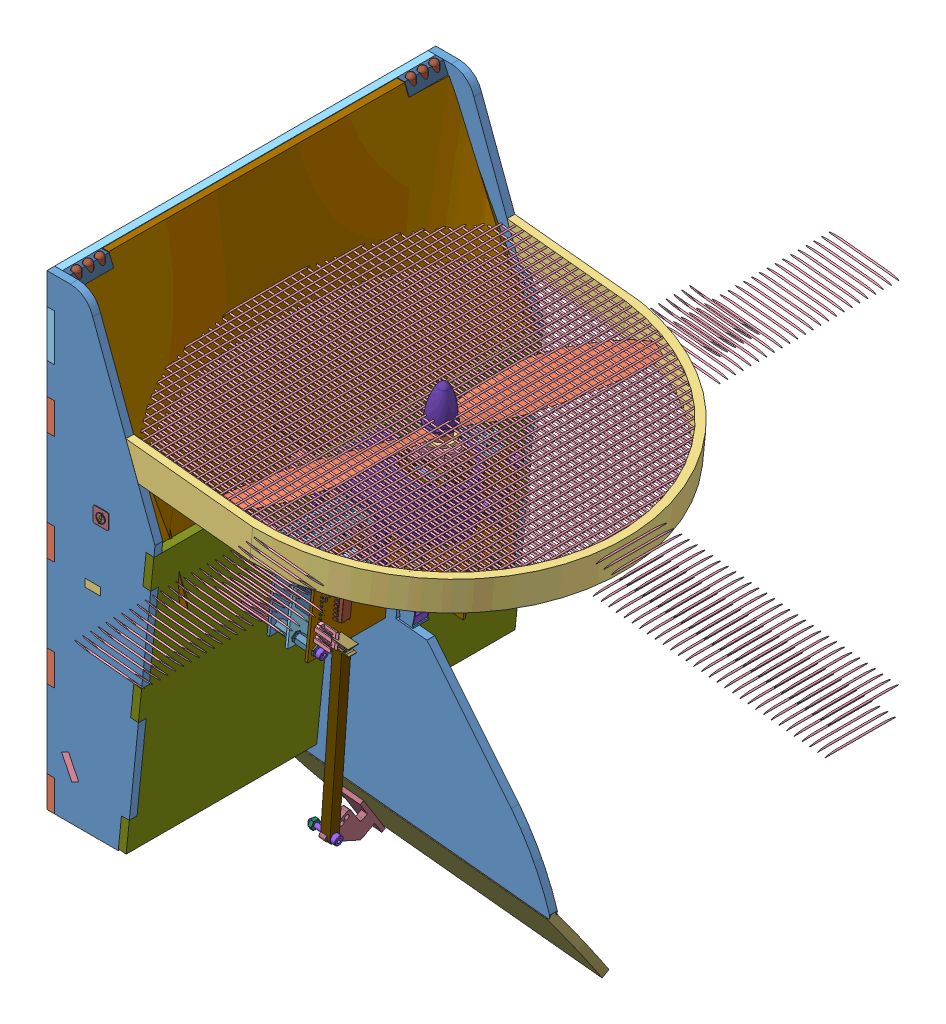
SolidWorks assembly AssTotaleSimu7, configuration Défaut. Lengths in mm. (continued)
Components (placement in the parent): (continued)
- AssStructSimu-1: AssStructSimu [Défaut] at (-125.7658 -1.8483 624.6548) x (1 0 0) z (0 0 -1) size (253.25 324.59 251.6) (continued)
  - AssCarte-1: AssCarte [Défaut] at (38.0121 147.1029 290.772) x (-0.101852 0.9948 0) z (0.9948 0.101852 0) size (66.52 130.57 98.72) (continued)
    - carte_onduleur_v3-1: carte_onduleur_v3 [Défaut] at (-131.8199 12.0892 20.7912) size (66.52 130.57 82.34) (continued)
      - U_DSPIC-1: U_DSPIC [Défaut] at (1.863 -2.61 0.803) size (7.92 35.56 7.75)
        - Open CASCADE STEP translator 6.8 1.17.1-1: Open CASCADE STEP translator 6.8 1.17.1 [Défaut] at origin size (7.92 35.56 7.75)
          - Body_1_4-1: Body_1_4 [Défaut] at (0 -0.2 4) x (1 0 0) z (0 -1 0) size (7.92 7.75 35.56)
      - C_DEC_DSPIC-1: C_DEC_DSPIC [Défaut] at (7.7 -8.8 -0.803) x (0 1 0) z (0 0 -1) size (2.34 1.04 0.5)
        - Open CASCADE STEP translator 6.8 1.6.1-1: Open CASCADE STEP translator 6.8 1.6.1 [Défaut] at origin size (2.34 1.04 0.5)
          - Body_1-1: Body_1 [Défaut] at origin size (2.29 1.04 0.43)
          - Pin_1-1: Pin_1 [Défaut] at (0.3048 0 0) x (-1 0 0) z (0 0 1) size (0.51 1.02 0.5)
          - Pin_2-1: Pin_2 [Défaut] at origin size (0.51 1.02 0.5)
      - IN-1: IN [Défaut] at (24.3 -5.3 0.803) x (0 1 0) z (0 0 1) size (10.21 15.56 26.9)
        - Open CASCADE STEP translator 6.8 1.19.1-1: Open CASCADE STEP translator 6.8 1.19.1 [Défaut] at origin size (10.21 15.56 26.9)
          - Body_1_3-1: Body_1_3 [Défaut] at (-13.5 1.8 3) x (0 1 0) z (1 0 0) size (15.56 26.9 10.21)
            - Imported-1: Imported [Défaut] at (2.0451 -4.5908 20.9802) size (8.6 15.9 10.16)
            - Imported-2: Imported [Défaut] at (-1.6683 9.1092 15.9802) x (0 0 1) z (-1 0 0) size (10.1 18.2 15.1)
              - Imported_2-1: Imported_2 [Défaut] at origin size (10.1 18.2 15.1)
              - Imported_3-1: Imported_3 [Défaut] at origin size (3.43 12.4 4.99)
              - Imported_4-1: Imported_4 [Défaut] at origin size (3.43 12.4 4.99)
              - Imported_5-1: Imported_5 [Défaut] at origin size (3.9 4.9 7)
              - Imported_6-1: Imported_6 [Défaut] at origin size (3.9 4.9 7)
              - Imported_7-1: Imported_7 [Défaut] at origin size (3.8 3.8 6.92)
              - Imported_8-1: Imported_8 [Défaut] at origin size (3.8 3.8 6.92)
              - Imported_9-1: Imported_9 [Défaut] at origin size (9 2.4 14.2)
      - CARTE_CMD-1: CARTE_CMD [Défaut] at (25 57.2 0.803) size (60.1 130 26.71)
        - Open CASCADE STEP translator 6.8 1.20.1-1: Open CASCADE STEP translator 6.8 1.20.1 [Défaut] at origin size (60.1 130 26.71)
          - Body_1_4-1: Body_1_4 [Défaut] at (-55 5 12) size (60.1 130 26.71)
            - 1_2-1: 1_2 [Défaut] at origin size (60.1 130 1.61)
            - 4-1: 4 [Défaut] at (23.6 -124.9 0.803) x (0 1 0) z (0 0 1) size (5 15.24 14.3)
              - =_[0_1_1_4]_2-1: =_[0_1_1_4]_2 [Défaut] at origin size (5 15.24 14.3)
                - 5-1: 5 [Défaut] at (0 -6.5 -13) x (0 1 0) z (0 0 -1) size (15.24 5 14.3)
            - 7-1: 7 [Défaut] at (23.6 -5 0.803) x (0 1 0) z (0 0 1) size (5 15.24 14.3)
              - =_[0_1_1_7]-1: =_[0_1_1_7] [Défaut] at origin size (5 15.24 14.3)
                - 5-1: 5 [Défaut] at (0 -6.5 -13) x (0 1 0) z (0 0 -1) size (15.24 5 14.3)
            - 10_2-1: 10_2 [Défaut] at (18.4 -115.6 0.803) size (25.4 7.92 7.75)
              - =_[0_1_1_9]-1: =_[0_1_1_9] [Défaut] at origin size (25.4 7.92 7.75)
                - 8-1: 8 [Défaut] at (11.2 4 0) x (0 1 0) z (1 0 0) size (7.92 7.75 25.4)
            - 13_2-1: 13_2 [Défaut] at (55.4 -114.7 0.803) x (-1 0 0) z (0 0 1) size (5 7.62 14.3)
              - =_[0_1_1_12]-1: =_[0_1_1_12] [Défaut] at origin size (5 7.62 14.3)
                - 11-1: 11 [Défaut] at (0 -2.5 11) x (0 -1 0) z (0 0 1) size (7.62 5 14.3)
            - 25-1: 25 [Défaut] at (56.9 -12.8 0.803) x (-1 0 0) z (0 0 1) size (16.02 47.26 11.05)
              - =_[0_1_1_15]_2-1: =_[0_1_1_15]_2 [Défaut] at origin size (16.02 47.26 11.05)
                - 23-1: 23 [Défaut] at (-36.5 21 4) x (0 -1 0) z (1 0 0) size (47.26 11.05 16.02)
                  - 14-1: 14 [Défaut] at (-7.4961 -1.5352 42.5833) size (42.58 6.55 16.01)
                  - 22-1: 22 [Défaut] at (19.3039 2.3748 37.905) x (-1 0 0) z (0 0 -1) size (10.36 6.14 15.24)
                    - 21-1: 21 [Défaut] at origin size (10.36 6.14 7.62)
                      - 19_2-1: 19_2 [Défaut] at origin size (10.36 6.14 2.54)
                        - 15-1: 15 [Défaut] at origin size (8.4 2.54 2.54)
                        - 16-1: 16 [Défaut] at (-0.0461 1.2682 1.27) x (0 0 -1) z (0.999998 -0.002105 0) size (1.95 5.07 7.58)
                      - 19_2-2: 19_2 [Défaut] at (0 0 -2.54) size (10.36 6.14 2.54)
                        - 15-1: 15 [Défaut] at origin size (8.4 2.54 2.54)
                        - 16-1: 16 [Défaut] at (-0.0461 1.2682 1.27) x (0 0 -1) z (0.999998 -0.002105 0) size (1.95 5.07 7.58)
                      - 19_2-3: 19_2 [Défaut] at (0 0 -5.08) size (10.36 6.14 2.54)
                        - 15-1: 15 [Défaut] at origin size (8.4 2.54 2.54)
                        - 16-1: 16 [Défaut] at (-0.0461 1.2682 1.27) x (0 0 -1) z (0.999998 -0.002105 0) size (1.95 5.07 7.58)
                    - 21-2: 21 [Défaut] at (0 0 -7.62) size (10.36 6.14 7.62)
                      - 19_2-1: 19_2 [Défaut] at origin size (10.36 6.14 2.54)
                        - 15-1: 15 [Défaut] at origin size (8.4 2.54 2.54)
                        - 16-1: 16 [Défaut] at (-0.0461 1.2682 1.27) x (0 0 -1) z (0.999998 -0.002105 0) size (1.95 5.07 7.58)
                      - 19_2-2: 19_2 [Défaut] at (0 0 -2.54) size (10.36 6.14 2.54)
                        - 15-1: 15 [Défaut] at origin size (8.4 2.54 2.54)
                        - 16-1: 16 [Défaut] at (-0.0461 1.2682 1.27) x (0 0 -1) z (0.999998 -0.002105 0) size (1.95 5.07 7.58)
                      - 19_2-3: 19_2 [Défaut] at (0 0 -5.08) size (10.36 6.14 2.54)
                        - 15-1: 15 [Défaut] at origin size (8.4 2.54 2.54)
                        - 16-1: 16 [Défaut] at (-0.0461 1.2682 1.27) x (0 0 -1) z (0.999998 -0.002105 0) size (1.95 5.07 7.58)
            - 31-1: 31 [Défaut] at (12.9 -104.5 0.803) size (6.76 3.64 4.37)
              - =_[0_1_1_24]-1: =_[0_1_1_24] [Défaut] at origin size (6.76 3.64 4.37)
                - 29-1: 29 [Défaut] at (-0.3 -2 0) size (6.76 3.64 4.37)
                  - =_[0_1_1_3]_3-1: =_[0_1_1_3]_3 [Défaut] at origin size (6 3.64 4.37)
                  - =_[0_1_1_4]_3-1: =_[0_1_1_4]_3 [Défaut] at origin size (0.38 1 0.67)
                  - =_[0_1_1_5]_3-1: =_[0_1_1_5]_3 [Défaut] at origin size (0.38 1 0.67)
            - 36-1: 36 [Défaut] at (28.6 -12.2 0.803) x (0 -1 0) z (0 0 1) size (2.34 1.04 0.5)
              - =_[0_1_1_30]-1: =_[0_1_1_30] [Défaut] at origin size (2.34 1.04 0.5)
                - 32_2-1: 32_2 [Défaut] at origin size (2.29 1.04 0.43)
                - 33_2-1: 33_2 [Défaut] at (0.3048 0 0) x (-1 0 0) z (0 0 1) size (0.51 1.02 0.5)
                - 34-1: 34 [Défaut] at origin size (0.51 1.02 0.5)
            - 38-1: 38 [Défaut] at (23.7 -12.2 0.803) x (0 -1 0) z (0 0 1) size (2.34 1.04 0.5)
              - =_[0_1_1_30]-1: =_[0_1_1_30] [Défaut] at origin size (2.34 1.04 0.5)
                - 32_2-1: 32_2 [Défaut] at origin size (2.29 1.04 0.43)
                - 33_2-1: 33_2 [Défaut] at (0.3048 0 0) x (-1 0 0) z (0 0 1) size (0.51 1.02 0.5)
                - 34-1: 34 [Défaut] at origin size (0.51 1.02 0.5)
            - 40_2-1: 40_2 [Défaut] at (26.2 -12.2 0.803) x (0 -1 0) z (0 0 1) size (2.34 1.04 0.5)
              - =_[0_1_1_30]-1: =_[0_1_1_30] [Défaut] at origin size (2.34 1.04 0.5)
                - 32_2-1: 32_2 [Défaut] at origin size (2.29 1.04 0.43)
                - 33_2-1: 33_2 [Défaut] at (0.3048 0 0) x (-1 0 0) z (0 0 1) size (0.51 1.02 0.5)
                - 34-1: 34 [Défaut] at origin size (0.51 1.02 0.5)
            - 42_2-1: 42_2 [Défaut] at (24.4 -119.2 0.803) size (2.34 1.04 0.5)
              - =_[0_1_1_30]-1: =_[0_1_1_30] [Défaut] at origin size (2.34 1.04 0.5)
                - 32_2-1: 32_2 [Défaut] at origin size (2.29 1.04 0.43)
                - 33_2-1: 33_2 [Défaut] at (0.3048 0 0) x (-1 0 0) z (0 0 1) size (0.51 1.02 0.5)
                - 34-1: 34 [Défaut] at origin size (0.51 1.02 0.5)
            - 45-1: 45 [Défaut] at (46.4 -125 0.803) size (5.08 5 14.3)
              - =_[0_1_1_38]-1: =_[0_1_1_38] [Défaut] at origin size (5.08 5 14.3)
                - 46-1: 46 [Défaut] at (1.2 0 11) size (5.08 5 14.3)
            - 48-1: 48 [Défaut] at (40.1 -125 0.803) size (5.08 5 14.3)
              - =_[0_1_1_41]-1: =_[0_1_1_41] [Défaut] at origin size (5.08 5 14.3)
                - 46-1: 46 [Défaut] at (1.2 0 11) size (5.08 5 14.3)
            - 51-1: 51 [Défaut] at (6.4 -119.9 0.803) x (0 1 0) z (0 0 1) size (15.24 2.54 7.37)
              - =_[0_1_1_43]-1: =_[0_1_1_43] [Défaut] at origin size (15.24 2.54 7.37)
                - 49_2-1: 49_2 [Défaut] at (6.5 0 0) x (1 0 0) z (0 -1 0) size (15.24 7.37 2.54)
            - 57_2-1: 57_2 [Défaut] at (50.8796 -121.1 -0.803) x (-1 0 0) z (0 0 -1) size (2.54 1.98 0.64)
              - =_[0_1_1_46]-1: =_[0_1_1_46] [Défaut] at origin size (2.54 1.98 0.64)
                - 52-1: 52 [Défaut] at origin size (2.54 1.14 0.58)
                - 53-1: 53 [Défaut] x (0 -1 0) z (0 0 1) size (0.43 0.51 0.38)
                - 54-1: 54 [Défaut] at (1.8796 1.8796 0) x (0 -1 0) z (0 0 1) size (0.43 0.51 0.38)
                - 55-1: 55 [Défaut] at (-0.9652 -2.8448 0) x (0 1 0) z (0 0 1) size (0.41 0.51 0.38)
            - 59_2-1: 59_2 [Défaut] at (43.6398 -120.995 -0.803) x (-1 0 0) z (0 0 -1) size (2.54 1.98 0.64)
              - =_[0_1_1_46]-1: =_[0_1_1_46] [Défaut] at origin size (2.54 1.98 0.64)
                - 52-1: 52 [Défaut] at origin size (2.54 1.14 0.58)
                - 53-1: 53 [Défaut] x (0 -1 0) z (0 0 1) size (0.43 0.51 0.38)
                - 54-1: 54 [Défaut] at (1.8796 1.8796 0) x (0 -1 0) z (0 0 1) size (0.43 0.51 0.38)
                - 55-1: 55 [Défaut] at (-0.9652 -2.8448 0) x (0 1 0) z (0 0 1) size (0.41 0.51 0.38)
            - 61_2-1: 61_2 [Défaut] at (47.6 -119.9 -0.803) x (-1 0 0) z (0 0 -1) size (2.34 1.04 0.5)
              - =_[0_1_1_30]-1: =_[0_1_1_30] [Défaut] at origin size (2.34 1.04 0.5)
                - 32_2-1: 32_2 [Défaut] at origin size (2.29 1.04 0.43)
                - 33_2-1: 33_2 [Défaut] at (0.3048 0 0) x (-1 0 0) z (0 0 1) size (0.51 1.02 0.5)
                - 34-1: 34 [Défaut] at origin size (0.51 1.02 0.5)
            - 63-1: 63 [Défaut] at (40.4 -119.9 -0.803) x (-1 0 0) z (0 0 -1) size (2.34 1.04 0.5)
              - =_[0_1_1_30]-1: =_[0_1_1_30] [Défaut] at origin size (2.34 1.04 0.5)
                - 32_2-1: 32_2 [Défaut] at origin size (2.29 1.04 0.43)
                - 33_2-1: 33_2 [Défaut] at (0.3048 0 0) x (-1 0 0) z (0 0 1) size (0.51 1.02 0.5)
                - 34-1: 34 [Défaut] at origin size (0.51 1.02 0.5)
            - 68-1: 68 [Défaut] at (47.7 -21.8 -0.803) x (0 1 0) z (0 0 -1) size (2.34 1.04 0.5)
              - =_[0_1_1_55]-1: =_[0_1_1_55] [Défaut] at origin size (2.34 1.04 0.5)
                - 64-1: 64 [Défaut] at origin size (2.29 1.04 0.43)
                - 65-1: 65 [Défaut] at (0.3048 0 0) x (-1 0 0) z (0 0 1) size (0.51 1.02 0.5)
                - 66-1: 66 [Défaut] at origin size (0.51 1.02 0.5)
            - 70-1: 70 [Défaut] at (47.6 -121.7 -0.803) x (-1 0 0) z (0 0 -1) size (2.34 1.04 0.5)
              - =_[0_1_1_30]-1: =_[0_1_1_30] [Défaut] at origin size (2.34 1.04 0.5)
                - 32_2-1: 32_2 [Défaut] at origin size (2.29 1.04 0.43)
                - 33_2-1: 33_2 [Défaut] at (0.3048 0 0) x (-1 0 0) z (0 0 1) size (0.51 1.02 0.5)
                - 34-1: 34 [Défaut] at origin size (0.51 1.02 0.5)
            - 72_2-1: 72_2 [Défaut] at (40.4 -121.5 -0.803) x (-1 0 0) z (0 0 -1) size (2.34 1.04 0.5)
              - =_[0_1_1_30]-1: =_[0_1_1_30] [Défaut] at origin size (2.34 1.04 0.5)
                - 32_2-1: 32_2 [Défaut] at origin size (2.29 1.04 0.43)
                - 33_2-1: 33_2 [Défaut] at (0.3048 0 0) x (-1 0 0) z (0 0 1) size (0.51 1.02 0.5)
                - 34-1: 34 [Défaut] at origin size (0.51 1.02 0.5)
            - 74_2-1: 74_2 [Défaut] at (47.7 -18.3 -0.803) x (0 1 0) z (0 0 -1) size (2.34 1.04 0.5)
              - =_[0_1_1_55]-1: =_[0_1_1_55] [Défaut] at origin size (2.34 1.04 0.5)
                - 64-1: 64 [Défaut] at origin size (2.29 1.04 0.43)
                - 65-1: 65 [Défaut] at (0.3048 0 0) x (-1 0 0) z (0 0 1) size (0.51 1.02 0.5)
                - 66-1: 66 [Défaut] at origin size (0.51 1.02 0.5)
            - 76_2-1: 76_2 [Défaut] at (45.5 -118.3 -0.803) x (1 0 0) z (0 0 -1) size (2.34 1.04 0.5)
              - =_[0_1_1_30]-1: =_[0_1_1_30] [Défaut] at origin size (2.34 1.04 0.5)
                - 32_2-1: 32_2 [Défaut] at origin size (2.29 1.04 0.43)
                - 33_2-1: 33_2 [Défaut] at (0.3048 0 0) x (-1 0 0) z (0 0 1) size (0.51 1.02 0.5)
                - 34-1: 34 [Défaut] at origin size (0.51 1.02 0.5)
            - 78_2-1: 78_2 [Défaut] at (38.2 -118.3 -0.803) x (1 0 0) z (0 0 -1) size (2.34 1.04 0.5)
              - =_[0_1_1_30]-1: =_[0_1_1_30] [Défaut] at origin size (2.34 1.04 0.5)
                - 32_2-1: 32_2 [Défaut] at origin size (2.29 1.04 0.43)
                - 33_2-1: 33_2 [Défaut] at (0.3048 0 0) x (-1 0 0) z (0 0 1) size (0.51 1.02 0.5)
                - 34-1: 34 [Défaut] at origin size (0.51 1.02 0.5)
            - 80_2-1: 80_2 [Défaut] at (28.6 -10.7 0.803) x (0 1 0) z (0 0 1) size (2.34 1.04 0.5)
              - =_[0_1_1_55]-1: =_[0_1_1_55] [Défaut] at origin size (2.34 1.04 0.5)
                - 64-1: 64 [Défaut] at origin size (2.29 1.04 0.43)
                - 65-1: 65 [Défaut] at (0.3048 0 0) x (-1 0 0) z (0 0 1) size (0.51 1.02 0.5)
                - 66-1: 66 [Défaut] at origin size (0.51 1.02 0.5)
            - 82_2-1: 82_2 [Défaut] at (23.7 -10.7 0.803) x (0 1 0) z (0 0 1) size (2.34 1.04 0.5)
              - =_[0_1_1_55]-1: =_[0_1_1_55] [Défaut] at origin size (2.34 1.04 0.5)
                - 64-1: 64 [Défaut] at origin size (2.29 1.04 0.43)
                - 65-1: 65 [Défaut] at (0.3048 0 0) x (-1 0 0) z (0 0 1) size (0.51 1.02 0.5)
                - 66-1: 66 [Défaut] at origin size (0.51 1.02 0.5)
            - 84-1: 84 [Défaut] at (26.2 -10.7 0.803) x (0 1 0) z (0 0 1) size (2.34 1.04 0.5)
              - =_[0_1_1_55]-1: =_[0_1_1_55] [Défaut] at origin size (2.34 1.04 0.5)
                - 64-1: 64 [Défaut] at origin size (2.29 1.04 0.43)
                - 65-1: 65 [Défaut] at (0.3048 0 0) x (-1 0 0) z (0 0 1) size (0.51 1.02 0.5)
                - 66-1: 66 [Défaut] at origin size (0.51 1.02 0.5)
            - 86-1: 86 [Défaut] at (23.0336 -119.2 0.803) x (-1 0 0) z (0 0 1) size (2.34 1.04 0.5)
              - =_[0_1_1_55]-1: =_[0_1_1_55] [Défaut] at origin size (2.34 1.04 0.5)
                - 64-1: 64 [Défaut] at origin size (2.29 1.04 0.43)
                - 65-1: 65 [Défaut] at (0.3048 0 0) x (-1 0 0) z (0 0 1) size (0.51 1.02 0.5)
                - 66-1: 66 [Défaut] at origin size (0.51 1.02 0.5)
            - 88-1: 88 [Défaut] at (14.1 -114.2 0.803) x (0 -1 0) z (0 0 1) size (2.34 1.04 0.5)
              - =_[0_1_1_55]-1: =_[0_1_1_55] [Défaut] at origin size (2.34 1.04 0.5)
                - 64-1: 64 [Défaut] at origin size (2.29 1.04 0.43)
                - 65-1: 65 [Défaut] at (0.3048 0 0) x (-1 0 0) z (0 0 1) size (0.51 1.02 0.5)
                - 66-1: 66 [Défaut] at origin size (0.51 1.02 0.5)
            - 90-1: 90 [Défaut] at (43.6 -107.8 -0.803) x (1 0 0) z (0 0 -1) size (2.34 1.04 0.5)
              - =_[0_1_1_55]-1: =_[0_1_1_55] [Défaut] at origin size (2.34 1.04 0.5)
                - 64-1: 64 [Défaut] at origin size (2.29 1.04 0.43)
                - 65-1: 65 [Défaut] at (0.3048 0 0) x (-1 0 0) z (0 0 1) size (0.51 1.02 0.5)
                - 66-1: 66 [Défaut] at origin size (0.51 1.02 0.5)
            - 92-1: 92 [Défaut] at (43.6 -106 -0.803) x (1 0 0) z (0 0 -1) size (2.34 1.04 0.5)
              - =_[0_1_1_55]-1: =_[0_1_1_55] [Défaut] at origin size (2.34 1.04 0.5)
                - 64-1: 64 [Défaut] at origin size (2.29 1.04 0.43)
                - 65-1: 65 [Défaut] at (0.3048 0 0) x (-1 0 0) z (0 0 1) size (0.51 1.02 0.5)
                - 66-1: 66 [Défaut] at origin size (0.51 1.02 0.5)
            - 175-1: 175 [Défaut] at (10 -21.7 0.803) x (0 -1 0) z (0 0 1) size (15 25.4 12.78)
              - =_[0_1_1_72]-1: =_[0_1_1_72] [Défaut] at origin size (15 25.4 12.78)
                - 173-1: 173 [Défaut] at (-1.4 -1 12) x (-1 0 0) z (0 1 0) size (15 12.78 25.4)
                  - board_1-1: board_1 [Défaut] at (-7.5 -1.57 12.5) size (15 1.57 25)
                  - hole_plating_20-1: hole_plating_20 [Défaut] at (-1.5 0 23.93) size (1.5 0.01 1.5)
                  - hole_plating_20-2: hole_plating_20 [Défaut] at (-1.5 0 21.39) size (1.5 0.01 1.5)
                  - hole_plating_20-3: hole_plating_20 [Défaut] at (-1.5 0 8.69) size (1.5 0.01 1.5)
                  - hole_plating_20-4: hole_plating_20 [Défaut] at (-1.5 -1.58 13.77) size (1.5 0.01 1.5)
                  - hole_plating_20-5: hole_plating_20 [Défaut] at (-1.5 0 16.31) size (1.5 0.01 1.5)
                  - hole_plating_20-6: hole_plating_20 [Défaut] at (-1.5 0 18.85) size (1.5 0.01 1.5)
                  - hole_plating_20-7: hole_plating_20 [Défaut] at (-1.5 0 13.77) size (1.5 0.01 1.5)
                  - hole_plating_20-8: hole_plating_20 [Défaut] at (-1.5 -1.58 11.23) size (1.5 0.01 1.5)
                  - hole_plating_20-9: hole_plating_20 [Défaut] at (-1.5 -1.58 18.85) size (1.5 0.01 1.5)
                  - hole_plating_20-10: hole_plating_20 [Défaut] at (-1.5 -1.58 6.15) size (1.5 0.01 1.5)
                  - hole_plating_20-11: hole_plating_20 [Défaut] at (-1.5 0 1.07) size (1.5 0.01 1.5)
                  - hole_plating_20-12: hole_plating_20 [Défaut] at (-1.5 -1.58 3.61) size (1.5 0.01 1.5)
                  - hole_plating_20-13: hole_plating_20 [Défaut] at (-1.5 -1.58 1.07) size (1.5 0.01 1.5)
                  - hole_plating_20-14: hole_plating_20 [Défaut] at (-1.5 -1.58 8.69) size (1.5 0.01 1.5)
                  - hole_plating_20-15: hole_plating_20 [Défaut] at (-1.5 -1.58 16.31) size (1.5 0.01 1.5)
                  - hole_plating_20-16: hole_plating_20 [Défaut] at (-1.5 0 11.23) size (1.5 0.01 1.5)
                  - hole_plating_20-17: hole_plating_20 [Défaut] at (-1.5 0 3.61) size (1.5 0.01 1.5)
                  - hole_plating_20-18: hole_plating_20 [Défaut] at (-1.5 -1.58 21.39) size (1.5 0.01 1.5)
                  - hole_plating_20-19: hole_plating_20 [Défaut] at (-1.5 0 6.15) size (1.5 0.01 1.5)
                  - hole_plating_20-20: hole_plating_20 [Défaut] at (-1.5 -1.58 23.93) size (1.5 0.01 1.5)
                  - Pin_Header_1x10_TH_Pitch_2.54mm_1-1: Pin_Header_1x10_TH_Pitch_2.54mm_1 [Défaut] at (-1.5 -1.5786 23.93) x (0 0 -1) z (0 -1 0) size (25.4 2.54 12.7)
                    - 124-1: 124 [Défaut] at origin size (25.4 2.54 2.8)
                      - =_[0_1_1_77]-1: =_[0_1_1_77] [Défaut] at origin size (2.54 2.54 2.8)
                      - =_[0_1_1_79]-1: =_[0_1_1_79] [Défaut] at origin size (2.54 2.54 2.8)
                      - =_[0_1_1_80]-1: =_[0_1_1_80] [Défaut] at origin size (2.54 2.54 2.8)
                      - =_[0_1_1_81]-1: =_[0_1_1_81] [Défaut] at origin size (2.54 2.54 2.8)
                      - =_[0_1_1_82]-1: =_[0_1_1_82] [Défaut] at origin size (2.54 2.54 2.8)
                      - =_[0_1_1_83]-1: =_[0_1_1_83] [Défaut] at origin size (2.54 2.54 2.8)
                      - =_[0_1_1_84]-1: =_[0_1_1_84] [Défaut] at origin size (2.54 2.54 2.8)
                      - =_[0_1_1_85]-1: =_[0_1_1_85] [Défaut] at origin size (2.54 2.54 2.8)
                      - =_[0_1_1_86]-1: =_[0_1_1_86] [Défaut] at origin size (2.54 2.54 2.8)
                      - =_[0_1_1_87]-1: =_[0_1_1_87] [Défaut] at origin size (2.54 2.54 2.8)
                    - 135-1: 135 [Défaut] at origin size (23.49 0.63 12.7)
                      - =_[0_1_1_88]-1: =_[0_1_1_88] [Défaut] at origin size (0.63 0.63 12.7)
                      - =_[0_1_1_90]-1: =_[0_1_1_90] [Défaut] at origin size (0.63 0.63 12.7)
                      - =_[0_1_1_91]-1: =_[0_1_1_91] [Défaut] at origin size (0.63 0.63 12.7)
                      - =_[0_1_1_92]-1: =_[0_1_1_92] [Défaut] at origin size (0.63 0.63 12.7)
                      - =_[0_1_1_93]-1: =_[0_1_1_93] [Défaut] at origin size (0.63 0.63 12.7)
                      - =_[0_1_1_94]-1: =_[0_1_1_94] [Défaut] at origin size (0.63 0.63 12.7)
                      - =_[0_1_1_95]-1: =_[0_1_1_95] [Défaut] at origin size (0.63 0.63 12.7)
                      - =_[0_1_1_96]-1: =_[0_1_1_96] [Défaut] at origin size (0.63 0.63 12.7)
                      - =_[0_1_1_97]-1: =_[0_1_1_97] [Défaut] at origin size (0.63 0.63 12.7)
                      - =_[0_1_1_98]-1: =_[0_1_1_98] [Défaut] at origin size (0.63 0.63 12.7)
                  - MPU-9250_1-1: MPU-9250_1 [Défaut] at (-8 0.05 12.5) x (-1 0 0) z (0 1 0) size (3 3 1.05)
                  - tantalum_10uF_1-1: tantalum_10uF_1 [Défaut] at (-13.167 0.1 10.9372) x (0 0 1) z (0 1 0) size (3.4 1.6 1.71)
                  - SOT23_5_1-1: SOT23_5_1 [Défaut] at (-7.475 -0.0136 21) x (0 0 1) z (0 1 0) size (3 3.2 0.92)
                  - RESC-0603_5-1: RESC-0603_5 [Défaut] at (-6.85 0 7.45) x (1 0 0) z (0 1 0) size (1.7 0.9 0.55)
                    - 143-1: 143 [Défaut] at origin size (1.7 0.9 0.55)
                      - =_[0_1_1_103]-1: =_[0_1_1_103] [Défaut] at origin size (0.4 0.9 0.53)
                      - =_[0_1_1_105]-1: =_[0_1_1_105] [Défaut] at origin size (0.4 0.9 0.53)
                      - =_[0_1_1_106]-1: =_[0_1_1_106] [Défaut] at origin size (1.64 0.9 0.52)
                    - 152-1: 152 [Défaut] at origin
                      - =_[0_1_1_107]-1: =_[0_1_1_107] [Défaut] at origin
                      - =_[0_1_1_109]-1: =_[0_1_1_109] [Défaut] at origin
                      - =_[0_1_1_110]-1: =_[0_1_1_110] [Défaut] at origin
                      - =_[0_1_1_111]-1: =_[0_1_1_111] [Défaut] at origin
                      - =_[0_1_1_112]-1: =_[0_1_1_112] [Défaut] at origin
                      - =_[0_1_1_113]-1: =_[0_1_1_113] [Défaut] at origin
                      - =_[0_1_1_114]-1: =_[0_1_1_114] [Défaut] at origin
                      - =_[0_1_1_115]-1: =_[0_1_1_115] [Défaut] at origin
                  - RESC-0603_5-2: RESC-0603_5 [Défaut] at (-9.85 0 16.05) x (1 0 0) z (0 1 0) size (1.7 0.9 0.55)
                    - 143-1: 143 [Défaut] at origin size (1.7 0.9 0.55)
                      - =_[0_1_1_103]-1: =_[0_1_1_103] [Défaut] at origin size (0.4 0.9 0.53)
                      - =_[0_1_1_105]-1: =_[0_1_1_105] [Défaut] at origin size (0.4 0.9 0.53)
                      - =_[0_1_1_106]-1: =_[0_1_1_106] [Défaut] at origin size (1.64 0.9 0.52)
                    - 152-1: 152 [Défaut] at origin
                      - =_[0_1_1_107]-1: =_[0_1_1_107] [Défaut] at origin
                      - =_[0_1_1_109]-1: =_[0_1_1_109] [Défaut] at origin
                      - =_[0_1_1_110]-1: =_[0_1_1_110] [Défaut] at origin
                      - =_[0_1_1_111]-1: =_[0_1_1_111] [Défaut] at origin
                      - =_[0_1_1_112]-1: =_[0_1_1_112] [Défaut] at origin
                      - =_[0_1_1_113]-1: =_[0_1_1_113] [Défaut] at origin
                      - =_[0_1_1_114]-1: =_[0_1_1_114] [Défaut] at origin
                      - =_[0_1_1_115]-1: =_[0_1_1_115] [Défaut] at origin
                  - RESC-0603_5-3: RESC-0603_5 [Défaut] at (-6.85 0 17.55) x (1 0 0) z (0 1 0) size (1.7 0.9 0.55)
                    - 143-1: 143 [Défaut] at origin size (1.7 0.9 0.55)
                      - =_[0_1_1_103]-1: =_[0_1_1_103] [Défaut] at origin size (0.4 0.9 0.53)
                      - =_[0_1_1_105]-1: =_[0_1_1_105] [Défaut] at origin size (0.4 0.9 0.53)
                      - =_[0_1_1_106]-1: =_[0_1_1_106] [Défaut] at origin size (1.64 0.9 0.52)
                    - 152-1: 152 [Défaut] at origin
                      - =_[0_1_1_107]-1: =_[0_1_1_107] [Défaut] at origin
                      - =_[0_1_1_109]-1: =_[0_1_1_109] [Défaut] at origin
                      - =_[0_1_1_110]-1: =_[0_1_1_110] [Défaut] at origin
                      - =_[0_1_1_111]-1: =_[0_1_1_111] [Défaut] at origin
                      - =_[0_1_1_112]-1: =_[0_1_1_112] [Défaut] at origin
                      - =_[0_1_1_113]-1: =_[0_1_1_113] [Défaut] at origin
                      - =_[0_1_1_114]-1: =_[0_1_1_114] [Défaut] at origin
                      - =_[0_1_1_115]-1: =_[0_1_1_115] [Défaut] at origin
                  - RESC-0603_5-4: RESC-0603_5 [Défaut] at (-6.85 0 16.05) x (1 0 0) z (0 1 0) size (1.7 0.9 0.55)
                    - 143-1: 143 [Défaut] at origin size (1.7 0.9 0.55)
                      - =_[0_1_1_103]-1: =_[0_1_1_103] [Défaut] at origin size (0.4 0.9 0.53)
                      - =_[0_1_1_105]-1: =_[0_1_1_105] [Défaut] at origin size (0.4 0.9 0.53)
                      - =_[0_1_1_106]-1: =_[0_1_1_106] [Défaut] at origin size (1.64 0.9 0.52)
                    - 152-1: 152 [Défaut] at origin
                      - =_[0_1_1_107]-1: =_[0_1_1_107] [Défaut] at origin
                      - =_[0_1_1_109]-1: =_[0_1_1_109] [Défaut] at origin
                      - =_[0_1_1_110]-1: =_[0_1_1_110] [Défaut] at origin
                      - =_[0_1_1_111]-1: =_[0_1_1_111] [Défaut] at origin
                      - =_[0_1_1_112]-1: =_[0_1_1_112] [Défaut] at origin
                      - =_[0_1_1_113]-1: =_[0_1_1_113] [Défaut] at origin
                      - =_[0_1_1_114]-1: =_[0_1_1_114] [Défaut] at origin
                      - =_[0_1_1_115]-1: =_[0_1_1_115] [Défaut] at origin
                  - RESC-0603_5-5: RESC-0603_5 [Défaut] at (-6.85 0 5.95) x (1 0 0) z (0 1 0) size (1.7 0.9 0.55)
                    - 143-1: 143 [Défaut] at origin size (1.7 0.9 0.55)
                      - =_[0_1_1_103]-1: =_[0_1_1_103] [Défaut] at origin size (0.4 0.9 0.53)
                      - =_[0_1_1_105]-1: =_[0_1_1_105] [Défaut] at origin size (0.4 0.9 0.53)
                      - =_[0_1_1_106]-1: =_[0_1_1_106] [Défaut] at origin size (1.64 0.9 0.52)
                    - 152-1: 152 [Défaut] at origin
                      - =_[0_1_1_107]-1: =_[0_1_1_107] [Défaut] at origin
                      - =_[0_1_1_109]-1: =_[0_1_1_109] [Défaut] at origin
                      - =_[0_1_1_110]-1: =_[0_1_1_110] [Défaut] at origin
                      - =_[0_1_1_111]-1: =_[0_1_1_111] [Défaut] at origin
                      - =_[0_1_1_112]-1: =_[0_1_1_112] [Défaut] at origin
                      - =_[0_1_1_113]-1: =_[0_1_1_113] [Défaut] at origin
                      - =_[0_1_1_114]-1: =_[0_1_1_114] [Défaut] at origin
                      - =_[0_1_1_115]-1: =_[0_1_1_115] [Défaut] at origin
                  - CAPC-0603-T0.9-BN_5-1: CAPC-0603-T0.9-BN_5 [Défaut] at (-9.85 0 8.95) x (1 0 0) z (0 1 0) size (1.7 0.9 0.9)
                    - =_[0_1_1_117]-1: =_[0_1_1_117] [Défaut] at origin size (1.7 0.9 0.9)
                    - 167-1: 167 [Défaut] at origin
                      - =_[0_1_1_118]-1: =_[0_1_1_118] [Défaut] at origin
                      - =_[0_1_1_120]-1: =_[0_1_1_120] [Défaut] at origin
                      - =_[0_1_1_121]-1: =_[0_1_1_121] [Défaut] at origin
                      - =_[0_1_1_122]-1: =_[0_1_1_122] [Défaut] at origin
                      - =_[0_1_1_123]-1: =_[0_1_1_123] [Défaut] at origin
                      - =_[0_1_1_124]-1: =_[0_1_1_124] [Défaut] at origin
                      - =_[0_1_1_125]-1: =_[0_1_1_125] [Défaut] at origin
                      - =_[0_1_1_126]-1: =_[0_1_1_126] [Défaut] at origin
                  - CAPC-0603-T0.9-BN_5-2: CAPC-0603-T0.9-BN_5 [Défaut] at (-6.85 0 8.95) x (1 0 0) z (0 1 0) size (1.7 0.9 0.9)
                    - =_[0_1_1_117]-1: =_[0_1_1_117] [Défaut] at origin size (1.7 0.9 0.9)
                    - 167-1: 167 [Défaut] at origin
                      - =_[0_1_1_118]-1: =_[0_1_1_118] [Défaut] at origin
                      - =_[0_1_1_120]-1: =_[0_1_1_120] [Défaut] at origin
                      - =_[0_1_1_121]-1: =_[0_1_1_121] [Défaut] at origin
                      - =_[0_1_1_122]-1: =_[0_1_1_122] [Défaut] at origin
                      - =_[0_1_1_123]-1: =_[0_1_1_123] [Défaut] at origin
                      - =_[0_1_1_124]-1: =_[0_1_1_124] [Défaut] at origin
                      - =_[0_1_1_125]-1: =_[0_1_1_125] [Défaut] at origin
                      - =_[0_1_1_126]-1: =_[0_1_1_126] [Défaut] at origin
                  - CAPC-0603-T0.9-BN_5-3: CAPC-0603-T0.9-BN_5 [Défaut] at (-6.85 0 19.05) x (1 0 0) z (0 1 0) size (1.7 0.9 0.9)
                    - =_[0_1_1_117]-1: =_[0_1_1_117] [Défaut] at origin size (1.7 0.9 0.9)
                    - 167-1: 167 [Défaut] at origin
                      - =_[0_1_1_118]-1: =_[0_1_1_118] [Défaut] at origin
                      - =_[0_1_1_120]-1: =_[0_1_1_120] [Défaut] at origin
                      - =_[0_1_1_121]-1: =_[0_1_1_121] [Défaut] at origin
                      - =_[0_1_1_122]-1: =_[0_1_1_122] [Défaut] at origin
                      - =_[0_1_1_123]-1: =_[0_1_1_123] [Défaut] at origin
                      - =_[0_1_1_124]-1: =_[0_1_1_124] [Défaut] at origin
                      - =_[0_1_1_125]-1: =_[0_1_1_125] [Défaut] at origin
                      - =_[0_1_1_126]-1: =_[0_1_1_126] [Défaut] at origin
                  - CAPC-0603-T0.9-BN_5-4: CAPC-0603-T0.9-BN_5 [Défaut] at (-9.85 0 7.45) x (1 0 0) z (0 1 0) size (1.7 0.9 0.9)
                    - =_[0_1_1_117]-1: =_[0_1_1_117] [Défaut] at origin size (1.7 0.9 0.9)
                    - 167-1: 167 [Défaut] at origin
                      - =_[0_1_1_118]-1: =_[0_1_1_118] [Défaut] at origin
                      - =_[0_1_1_120]-1: =_[0_1_1_120] [Défaut] at origin
                      - =_[0_1_1_121]-1: =_[0_1_1_121] [Défaut] at origin
                      - =_[0_1_1_122]-1: =_[0_1_1_122] [Défaut] at origin
                      - =_[0_1_1_123]-1: =_[0_1_1_123] [Défaut] at origin
                      - =_[0_1_1_124]-1: =_[0_1_1_124] [Défaut] at origin
                      - =_[0_1_1_125]-1: =_[0_1_1_125] [Défaut] at origin
                      - =_[0_1_1_126]-1: =_[0_1_1_126] [Défaut] at origin
                  - CAPC-0603-T0.9-BN_5-5: CAPC-0603-T0.9-BN_5 [Défaut] at (-9.85 0 17.55) x (1 0 0) z (0 1 0) size (1.7 0.9 0.9)
                    - =_[0_1_1_117]-1: =_[0_1_1_117] [Défaut] at origin size (1.7 0.9 0.9)
                    - 167-1: 167 [Défaut] at origin
                      - =_[0_1_1_118]-1: =_[0_1_1_118] [Défaut] at origin
                      - =_[0_1_1_120]-1: =_[0_1_1_120] [Défaut] at origin
                      - =_[0_1_1_121]-1: =_[0_1_1_121] [Défaut] at origin
                      - =_[0_1_1_122]-1: =_[0_1_1_122] [Défaut] at origin
                      - =_[0_1_1_123]-1: =_[0_1_1_123] [Défaut] at origin
                      - =_[0_1_1_124]-1: =_[0_1_1_124] [Défaut] at origin
                      - =_[0_1_1_125]-1: =_[0_1_1_125] [Défaut] at origin
                      - =_[0_1_1_126]-1: =_[0_1_1_126] [Défaut] at origin
            - 177-1: 177 [Défaut] at (52.1 -16.5 -0.803) x (1 0 0) z (0 0 -1) size (2.34 1.04 0.5)
              - =_[0_1_1_30]-1: =_[0_1_1_30] [Défaut] at origin size (2.34 1.04 0.5)
                - 32_2-1: 32_2 [Défaut] at origin size (2.29 1.04 0.43)
                - 33_2-1: 33_2 [Défaut] at (0.3048 0 0) x (-1 0 0) z (0 0 1) size (0.51 1.02 0.5)
                - 34-1: 34 [Défaut] at origin size (0.51 1.02 0.5)
            - 179-1: 179 [Défaut] at (22.5336 -121.5 -0.803) x (-1 0 0) z (0 0 -1) size (2.34 1.04 0.5)
              - =_[0_1_1_30]-1: =_[0_1_1_30] [Défaut] at origin size (2.34 1.04 0.5)
                - 32_2-1: 32_2 [Défaut] at origin size (2.29 1.04 0.43)
                - 33_2-1: 33_2 [Défaut] at (0.3048 0 0) x (-1 0 0) z (0 0 1) size (0.51 1.02 0.5)
                - 34-1: 34 [Défaut] at origin size (0.51 1.02 0.5)
            - 181-1: 181 [Défaut] at (48.6 -127 -0.803) x (-1 0 0) z (0 0 -1) size (2.34 1.04 0.5)
              - =_[0_1_1_30]-1: =_[0_1_1_30] [Défaut] at origin size (2.34 1.04 0.5)
                - 32_2-1: 32_2 [Défaut] at origin size (2.29 1.04 0.43)
                - 33_2-1: 33_2 [Défaut] at (0.3048 0 0) x (-1 0 0) z (0 0 1) size (0.51 1.02 0.5)
                - 34-1: 34 [Défaut] at origin size (0.51 1.02 0.5)
            - 183-1: 183 [Défaut] at (26.0189 -121.5 0.803) size (2.34 1.04 0.5)
              - =_[0_1_1_30]-1: =_[0_1_1_30] [Défaut] at origin size (2.34 1.04 0.5)
                - 32_2-1: 32_2 [Défaut] at origin size (2.29 1.04 0.43)
                - 33_2-1: 33_2 [Défaut] at (0.3048 0 0) x (-1 0 0) z (0 0 1) size (0.51 1.02 0.5)
                - 34-1: 34 [Défaut] at origin size (0.51 1.02 0.5)
            - 185-1: 185 [Défaut] at (30.3664 -19 -0.803) x (1 0 0) z (0 0 -1) size (2.34 1.04 0.5)
              - =_[0_1_1_30]-1: =_[0_1_1_30] [Défaut] at origin size (2.34 1.04 0.5)
                - 32_2-1: 32_2 [Défaut] at origin size (2.29 1.04 0.43)
                - 33_2-1: 33_2 [Défaut] at (0.3048 0 0) x (-1 0 0) z (0 0 1) size (0.51 1.02 0.5)
                - 34-1: 34 [Défaut] at origin size (0.51 1.02 0.5)
            - 187-1: 187 [Défaut] at (51.7 -114.3 -0.803) x (0 1 0) z (0 0 -1) size (2.34 1.04 0.5)
              - =_[0_1_1_30]-1: =_[0_1_1_30] [Défaut] at origin size (2.34 1.04 0.5)
                - 32_2-1: 32_2 [Défaut] at origin size (2.29 1.04 0.43)
                - 33_2-1: 33_2 [Défaut] at (0.3048 0 0) x (-1 0 0) z (0 0 1) size (0.51 1.02 0.5)
                - 34-1: 34 [Défaut] at origin size (0.51 1.02 0.5)
            - 189-1: 189 [Défaut] at (50 -114.3 -0.803) x (0 1 0) z (0 0 -1) size (2.34 1.04 0.5)
              - =_[0_1_1_30]-1: =_[0_1_1_30] [Défaut] at origin size (2.34 1.04 0.5)
                - 32_2-1: 32_2 [Défaut] at origin size (2.29 1.04 0.43)
                - 33_2-1: 33_2 [Défaut] at (0.3048 0 0) x (-1 0 0) z (0 0 1) size (0.51 1.02 0.5)
                - 34-1: 34 [Défaut] at origin size (0.51 1.02 0.5)
      - C2_1-1: C2_1 [Défaut] at (-20.6984 1.8 -0.803) x (1 0 0) z (0 0 -1) size (2.34 1.04 0.5)
        - Open CASCADE STEP translator 6.8 1.6.1-1: Open CASCADE STEP translator 6.8 1.6.1 [Défaut] at origin size (2.34 1.04 0.5)
          - Body_1-1: Body_1 [Défaut] at origin size (2.29 1.04 0.43)
          - Pin_1-1: Pin_1 [Défaut] at (0.3048 0 0) x (-1 0 0) z (0 0 1) size (0.51 1.02 0.5)
          - Pin_2-1: Pin_2 [Défaut] at origin size (0.51 1.02 0.5)
      - C2_2-1: C2_2 [Défaut] at (-24.2 1.8 -0.803) x (1 0 0) z (0 0 -1) size (2.34 1.04 0.5)
        - Open CASCADE STEP translator 6.8 1.6.1-1: Open CASCADE STEP translator 6.8 1.6.1 [Défaut] at origin size (2.34 1.04 0.5)
          - Body_1-1: Body_1 [Défaut] at origin size (2.29 1.04 0.43)
          - Pin_1-1: Pin_1 [Défaut] at (0.3048 0 0) x (-1 0 0) z (0 0 1) size (0.51 1.02 0.5)
          - Pin_2-1: Pin_2 [Défaut] at origin size (0.51 1.02 0.5)
      - C3_1-1: C3_1 [Défaut] at (-20.9176 -12.8 -0.803) x (1 0 0) z (0 0 -1) size (2.34 1.04 0.5)
        - Open CASCADE STEP translator 6.8 1.6.1-1: Open CASCADE STEP translator 6.8 1.6.1 [Défaut] at origin size (2.34 1.04 0.5)
          - Body_1-1: Body_1 [Défaut] at origin size (2.29 1.04 0.43)
          - Pin_1-1: Pin_1 [Défaut] at (0.3048 0 0) x (-1 0 0) z (0 0 1) size (0.51 1.02 0.5)
          - Pin_2-1: Pin_2 [Défaut] at origin size (0.51 1.02 0.5)
      - C3_2-1: C3_2 [Défaut] at (-24.4 -12.8 -0.803) x (1 0 0) z (0 0 -1) size (2.34 1.04 0.5)
        - Open CASCADE STEP translator 6.8 1.6.1-1: Open CASCADE STEP translator 6.8 1.6.1 [Défaut] at origin size (2.34 1.04 0.5)
          - Body_1-1: Body_1 [Défaut] at origin size (2.29 1.04 0.43)
          - Pin_1-1: Pin_1 [Défaut] at (0.3048 0 0) x (-1 0 0) z (0 0 1) size (0.51 1.02 0.5)
          - Pin_2-1: Pin_2 [Défaut] at origin size (0.51 1.02 0.5)
      - D_CUR-1: D_CUR [Défaut] at (-12.4432 3.85 -0.803) x (0 -1 0) z (0 0 -1) size (2.7 5.2 1.11)
        - Open CASCADE STEP translator 6.8 1.25.1-1: Open CASCADE STEP translator 6.8 1.25.1 [Défaut] at origin size (2.7 5.2 1.11)
          - Body_1_5-1: Body_1_5 [Défaut] at (1.2 -4 0) x (0 1 0) z (0 0 1) size (5.2 2.7 1.11)
            - =_[0_1_1_3]_4-1: =_[0_1_1_3]_4 [Défaut] at origin size (0.39 0.64 0.01)
            - =_[0_1_1_4]_4-1: =_[0_1_1_4]_4 [Défaut] at origin size (0.6 1.9 0.2)
            - =_[0_1_1_5]_4-1: =_[0_1_1_5]_4 [Défaut] at origin size (0.21 0.08 0.01)
            - =_[0_1_1_6]_2-1: =_[0_1_1_6]_2 [Défaut] at origin size (0.6 1.9 0.2)
            - =_[0_1_1_7]_2-1: =_[0_1_1_7]_2 [Défaut] at origin size (0.46 0.68 0.01)
            - =_[0_1_1_8]_2-1: =_[0_1_1_8]_2 [Défaut] at origin size (0.38 0.66 0.01)
            - =_[0_1_1_9]-1: =_[0_1_1_9] [Défaut] at origin size (0.2 0.62 0.01)
            - =_[0_1_1_10]-1: =_[0_1_1_10] [Défaut] at origin size (4 2.7 1.1)
            - =_[0_1_1_11]-1: =_[0_1_1_11] [Défaut] at origin size (0.46 0.63 0.01)
            - =_[0_1_1_12]-1: =_[0_1_1_12] [Défaut] at origin size (0.56 0.68 0.01)
      - RC1_1-1: RC1_1 [Défaut] at (-20.7176 8.1 -0.803) x (1 0 0) z (0 0 -1) size (2.34 1.04 0.5)
        - Open CASCADE STEP translator 6.8 1.12.1-1: Open CASCADE STEP translator 6.8 1.12.1 [Défaut] at origin size (2.34 1.04 0.5)
          - Body_1_3-1: Body_1_3 [Défaut] at origin size (2.29 1.04 0.43)
          - Pin_1_2-1: Pin_1_2 [Défaut] at (0.3048 0 0) x (-1 0 0) z (0 0 1) size (0.51 1.02 0.5)
          - Pin_2_2-1: Pin_2_2 [Défaut] at origin size (0.51 1.02 0.5)
      - RC1_2-1: RC1_2 [Défaut] at (-22 8.1 -0.803) x (-1 0 0) z (0 0 -1) size (2.34 1.04 0.5)
        - Open CASCADE STEP translator 6.8 1.12.1-1: Open CASCADE STEP translator 6.8 1.12.1 [Défaut] at origin size (2.34 1.04 0.5)
          - Body_1_3-1: Body_1_3 [Défaut] at origin size (2.29 1.04 0.43)
          - Pin_1_2-1: Pin_1_2 [Défaut] at (0.3048 0 0) x (-1 0 0) z (0 0 1) size (0.51 1.02 0.5)
          - Pin_2_2-1: Pin_2_2 [Défaut] at origin size (0.51 1.02 0.5)
      - RC2_1-1: RC2_1 [Défaut] at (-20.716 0.243 -0.803) x (1 0 0) z (0 0 -1) size (2.34 1.04 0.5)
        - Open CASCADE STEP translator 6.8 1.12.1-1: Open CASCADE STEP translator 6.8 1.12.1 [Défaut] at origin size (2.34 1.04 0.5)
          - Body_1_3-1: Body_1_3 [Défaut] at origin size (2.29 1.04 0.43)
          - Pin_1_2-1: Pin_1_2 [Défaut] at (0.3048 0 0) x (-1 0 0) z (0 0 1) size (0.51 1.02 0.5)
          - Pin_2_2-1: Pin_2_2 [Défaut] at origin size (0.51 1.02 0.5)
      - RC2_2-1: RC2_2 [Défaut] at (-22 0.18 -0.803) x (-1 0 0) z (0 0 -1) size (2.34 1.04 0.5)
        - Open CASCADE STEP translator 6.8 1.12.1-1: Open CASCADE STEP translator 6.8 1.12.1 [Défaut] at origin size (2.34 1.04 0.5)
          - Body_1_3-1: Body_1_3 [Défaut] at origin size (2.29 1.04 0.43)
          - Pin_1_2-1: Pin_1_2 [Défaut] at (0.3048 0 0) x (-1 0 0) z (0 0 1) size (0.51 1.02 0.5)
